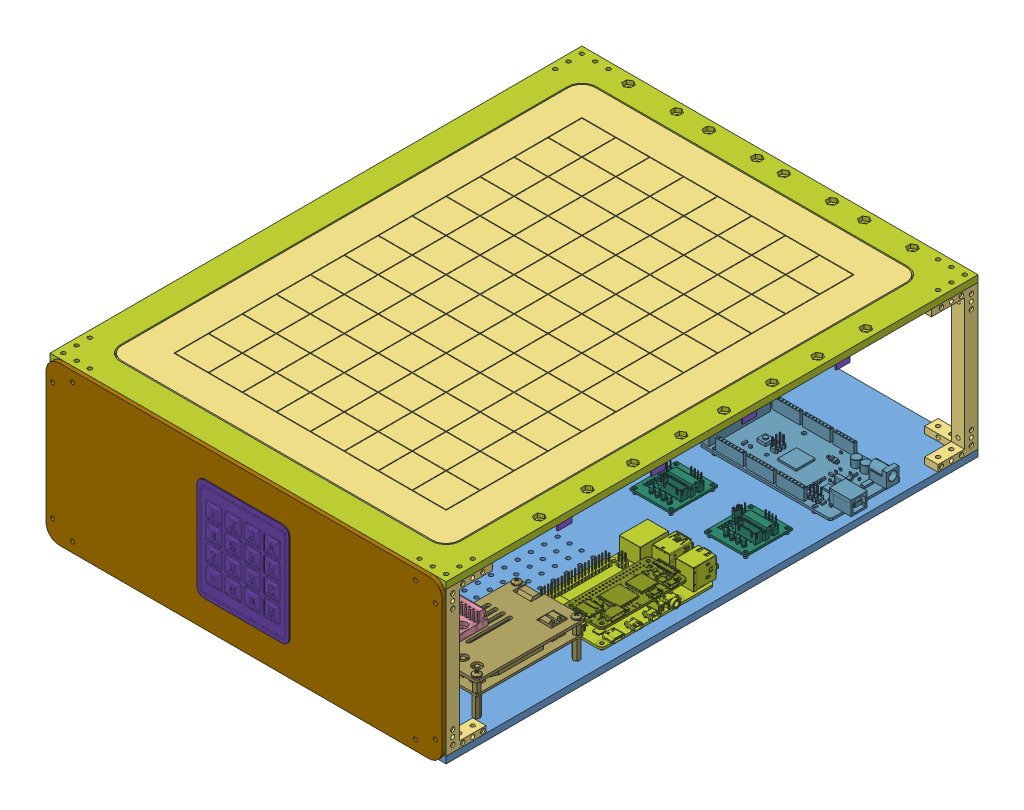
SolidWorks assembly FinalAssembly, configuration Default. Lengths in mm.
Overall size (297.5 118.5 403.99).
41 component instances, 27 part files, 115 mates.
Components (placement in the parent):
- Base-1: Base [Default] at (-28.1272 210.7626 518.1908) size (297.5 5 399.5)
- GearTrackLongAxisSinglePiece-1: GearTrackLongAxisSinglePiece [Default] at (155.3139 84.2058 503.2065) x (1 0 0) z (0 1 0) size (28 365.38 12.5)
- CornerJoin-1: CornerJoin [Default] at (-28.1272 215.7626 518.1908) size (35 108.5 35)
- CornerJoin-2: CornerJoin [Default] at (-28.1272 215.7626 118.6908) x (0 0 1) z (-1 0 0) size (35 108.5 35)
- CornerJoin-3: CornerJoin [Default] at (269.3728 215.7626 518.1908) x (0 0 -1) z (1 0 0) size (35 108.5 35)
- CornerJoin-4: CornerJoin [Default] at (269.3728 215.7626 118.6908) x (-1 0 0) z (0 0 -1) size (35 108.5 35)
- GearTrackShortAxisSinglePiece-1: GearTrackShortAxisSinglePiece [Default] at (251.3609 131.6956 442.9057) x (0 0 -1) z (0 1 0) size (28 245.31 12.5)
- AxisCartMount-1: AxisCartMount [Default] at (141.6223 251.1626 455.8667) x (-1 0 0) z (0 0 -1) size (154 5 33)
- ShortAxisLimitMount-1: ShortAxisLimitMount [Default] at (-19.5822 261.1626 458.0758) x (0 0 1) z (0 1 0) size (28 20 33)
- NewTopMount-1: NewTopMount [Default] at (-28.1272 324.2626 118.6908) x (0 0 1) z (-1 0 0) size (399.5 5 297.5)
- MotorCartMount-1: MotorCartMount [Default] at (63.6531 231.1626 374.4235) x (1 0 0) z (0 -1 0) size (44.96 33 30.65)
- MotorCartMount-2: MotorCartMount [Default] at (116.278 271.5626 415.1046) x (0 0 1) z (0 -1 0) size (44.96 33 30.65)
- EndEffectorMountV2-1: EndEffectorMountV2 [Default] at (1.8349 289.5626 493.0738) size (39 25 47)
- LCD_1602-1: LCD_1602 [Default] at (48.0597 363.4765 514.5115) x (1 0 0) z (0 -1 0) size (80 17 36)
- MagneticRod-1: MagneticRod [Default] at (18.3378 322.4583 471.3738) x (-1 0 0) z (0 0 1) size (5.8 23.9 5.8)
- ZK-JVA-12KX-1: ZK-JVA-12KX [Default] at (276.4205 168.0705 467.5621) x (0 0 -1) z (0 1 0) size (82 52 29.13)
- 28BYJ-48 5V Stepper Motor-1: 28BYJ-48 5V Stepper Motor [Default] at (120.624 250.1626 471.8089) x (1 0 0) z (0 -1 0) size (42 52.5 29)
- 28BYJ-48 5V Stepper Motor-2: 28BYJ-48 5V Stepper Motor [Default] at (18.8927 290.5626 472.0755) x (0 0 1) z (0 -1 0) size (42 52.5 29)
- ArduinoMega-1: ArduinoMega [Default] at (212.2228 219.4136 196.4827) x (1 0 0) z (0 -1 0) size (107.95 53.42 12.95)
- ULN2003-1: ULN2003 [Default] at (223.3728 217.7626 278.1908) x (1 0 0) z (0 1 0) size (31 35 11.29)
- ULN2003-2: ULN2003 [Default] at (167.3728 217.7626 278.1908) x (1 0 0) z (0 1 0) size (31 35 11.29)
- Raspberry Pi Zero 2 W-1: Raspberry Pi Zero 2 W [Default] at (246.3728 231.5626 360.6908) x (0 0 -1) z (1 0 0) size (65.8 5.05 30.58)
- keypad-16KeyMembrane-1: keypad-16KeyMembrane [Default] at (120.6223 270.0105 522.0036) x (1 0 0) z (0 -1 0) size (68.96 10.64 77.9)
- HK15178B-1: HK15178B [Default] at (24.2327 310.5583 503.0738) x (1 0 0) z (0 1 0) size (37.75 30.2 12)
- limit switch-1: limit switch [Default] at (-9.5822 279.1626 463.0758) x (-1 0 0) z (0 0 -1) size (26 20 11)
- limit switch-2: limit switch [Default] at (139.3728 240.7626 500.1908) x (0 0 1) z (-1 0 0) size (26 20 11)
- LongAxisLimitMount-1: LongAxisLimitMount [Default] at (134.3728 222.7626 510.1908) x (1 0 0) z (0 1 0) size (15 15 35)
- Board-2: Board [Default] at (-6.1272 326.2626 496.1908) size (253.5 3 355.5)
- RodAttach-1: RodAttach [Default] at (18.3378 322.5583 471.3738) x (0 0 1) z (1 0 0) size (14.5 24 9)
- LED-1: LED [Default] at (211.8357 326.4426 224.6643) x (0 0 -1) z (1 0 0) size (3.38 1.82 10.82)
- HallEffect-1: HallEffect [Default] at (207.8504 326.8526 230.6307) size (3.92 1.41 7.9)
- Raspberry Pi 4 Model B(CHIP SHORT REPLACEMENT)-1: Raspberry Pi 4 Model B(CHIP SHORT REPLACEMENT) [Default] at (233.3728 218.5626 350.6908) x (0 0 -1) z (1 0 0) size (89 19.92 58.4)
- 16ChannelMux-1: 16ChannelMux [Default] at (11.8728 324.2626 140.6908) x (0 0 -1) z (-1 0 0) size (17 9.94 40.4)
- 16ChannelMux-2: 16ChannelMux [Default] at (247.3728 324.2626 264.0908) x (1 0 0) z (0 0 -1) size (17 9.94 40.4)
- 16ChannelMux-3: 16ChannelMux [Default] at (72.2728 324.2626 140.6908) x (0 0 -1) z (-1 0 0) size (17 9.94 40.4)
- 16ChannelMux-4: 16ChannelMux [Default] at (128.5728 324.2626 140.6908) x (0 0 -1) z (-1 0 0) size (17 9.94 40.4)
- 16ChannelMux-5: 16ChannelMux [Default] at (247.3728 324.2626 402.7908) x (1 0 0) z (0 0 -1) size (17 9.94 40.4)
- 16ChannelMux-6: 16ChannelMux [Default] at (247.3728 324.2626 332.3908) x (1 0 0) z (0 0 -1) size (17 9.94 40.4)
- 16ChannelMux-7: 16ChannelMux [Default] at (247.3728 324.2626 193.6908) x (1 0 0) z (0 0 -1) size (17 9.94 40.4)
- 16ChannelMux-8: 16ChannelMux [Default] at (188.9728 324.2626 140.6908) x (0 0 -1) z (-1 0 0) size (17 9.94 40.4)
- InterfaceWall-1: InterfaceWall [Default] at (-28.1272 210.7626 518.1908) size (297.5 118.5 3)
Mates (geometry in assembly coordinates):
- Coincident1: coincident anti-aligned: plane of Base-1 through (-28.1272 215.7626 518.1908) normal (0 1 0); plane of GearTrackLongAxisSinglePiece-1 through (20.6226 215.7626 295.7853) normal (0 -1 0)
- Concentric1: concentric aligned: circle of Base-1; circle of GearTrackLongAxisSinglePiece-1
- Parallel2: parallel aligned: plane of Base-1 through (269.3728 215.7626 518.1908) normal (1 0 0); plane of GearTrackLongAxisSinglePiece-1 through (134.6203 215.7626 535.9174) normal (1 0 0)
- Coincident4: coincident anti-aligned: plane of Base-1 through (-28.1272 215.7626 518.1908) normal (0 1 0); plane of CornerJoin-1 through (-28.1272 215.7626 518.1908) normal (0 -1 0)
- Coincident6: coincident aligned: plane of Base-1 through (-28.1272 215.7626 518.1908) normal (0 0 1); plane of CornerJoin-1 through (-28.1272 225.7626 518.1908) normal (0 0 1)
- Coincident7: coincident aligned: plane of Base-1 through (-28.1272 215.7626 518.1908) normal (-1 0 0); plane of CornerJoin-1 through (-28.1272 225.7626 518.1908) normal (-1 0 0)
- Coincident8: coincident aligned: plane of Base-1 through (-28.1272 215.7626 518.1908) normal (-1 0 0); plane of CornerJoin-2 through (-28.1272 225.7626 118.6908) normal (-1 0 0)
- Coincident9: coincident anti-aligned: plane of Base-1 through (-28.1272 215.7626 518.1908) normal (0 1 0); plane of CornerJoin-2 through (-28.1272 215.7626 118.6908) normal (0 -1 0)
- Coincident10: coincident aligned: plane of Base-1 through (-28.1272 215.7626 118.6908) normal (0 0 -1); plane of CornerJoin-2 through (-28.1272 225.7626 118.6908) normal (0 0 -1)
- Coincident11: coincident anti-aligned: plane of Base-1 through (-28.1272 215.7626 518.1908) normal (0 1 0); plane of CornerJoin-3 through (269.3728 215.7626 518.1908) normal (0 -1 0)
- Coincident12: coincident aligned: plane of Base-1 through (-28.1272 215.7626 518.1908) normal (0 0 1); plane of CornerJoin-3 through (269.3728 225.7626 518.1908) normal (0 0 1)
- Coincident13: coincident aligned: plane of Base-1 through (269.3728 215.7626 518.1908) normal (1 0 0); plane of CornerJoin-3 through (269.3728 225.7626 518.1908) normal (1 0 0)
- Coincident14: coincident anti-aligned: plane of Base-1 through (-28.1272 215.7626 518.1908) normal (0 1 0); plane of CornerJoin-4 through (269.3728 215.7626 118.6908) normal (0 -1 0)
- Coincident15: coincident aligned: plane of Base-1 through (-28.1272 215.7626 118.6908) normal (0 0 -1); plane of CornerJoin-4 through (269.3728 225.7626 118.6908) normal (0 0 -1)
- Coincident16: coincident aligned: plane of Base-1 through (269.3728 215.7626 518.1908) normal (1 0 0); plane of CornerJoin-4 through (269.3728 225.7626 118.6908) normal (1 0 0)
- Coincident17: coincident anti-aligned: plane of CornerJoin-1 through (-28.1272 324.2626 518.1908) normal (0 1 0); plane of NewTopMount-1 through (-28.1272 324.2626 118.6908) normal (0 -1 0)
- Coincident18: coincident aligned: plane of CornerJoin-3 through (269.3728 225.7626 518.1908) normal (0 0 1); plane of NewTopMount-1 through (-28.1272 329.2626 518.1908) normal (0 0 1)
- Coincident19: coincident aligned: plane of CornerJoin-3 through (269.3728 225.7626 518.1908) normal (1 0 0); plane of NewTopMount-1 through (269.3728 329.2626 118.6908) normal (1 0 0)
- Coincident24: coincident anti-aligned: plane of GearTrackLongAxisSinglePiece-1 through (20.6226 228.2626 535.9174) normal (0 1 0); plane of MotorCartMount-1 through (63.6531 228.2626 374.4235) normal (0 -1 0)
- Distance3: distance = 7 mm aligned: plane of GearTrackLongAxisSinglePiece-1 through (106.6223 215.7626 535.9174) normal (-1 0 0); plane of MotorCartMount-1 through (99.6223 231.1626 374.4235) normal (-1 0 0)
- Coincident26: coincident anti-aligned: plane of AxisCartMount-1 through (141.6223 251.1626 455.8667) normal (0 -1 0); plane of MotorCartMount-1 through (63.6531 251.1626 374.4235) normal (0 1 0)
- Coincident27: coincident aligned: plane of AxisCartMount-1 through (141.6223 256.1626 455.8667) normal (0 0 -1); plane of MotorCartMount-1 through (63.6531 231.1626 455.8667) normal (0 0 -1)
- Concentric2: concentric aligned: cylinder of AxisCartMount-1 through (137.8723 247.1626 460.3667) axis (0 1 0) radius 1.65; cylinder of MotorCartMount-1 through (137.8723 212.1626 460.3667) axis (0 1 0) radius 1.65
- Coincident29: coincident anti-aligned: plane of GearTrackShortAxisSinglePiece-1 through (0.5498 256.1626 486.0738) normal (0 -1 0); plane of AxisCartMount-1 through (141.6223 256.1626 455.8667) normal (0 1 0)
- Concentric5: concentric aligned: circle of GearTrackShortAxisSinglePiece-1; circle of AxisCartMount-1
- Parallel5: parallel aligned: plane of GearTrackShortAxisSinglePiece-1 through (0.5498 260.9126 486.0738) normal (0 0 1); plane of AxisCartMount-1 through (141.6223 256.1626 488.8667) normal (0 0 1)
- Coincident34: coincident anti-aligned: plane of GearTrackShortAxisSinglePiece-1 through (0.4178 256.1626 572.0736) normal (-1 0 0); plane of ShortAxisLimitMount-1 through (0.4178 261.1626 458.0758) normal (1 0 0)
- Coincident35: coincident aligned: plane of GearTrackShortAxisSinglePiece-1 through (157.8602 256.1626 572.0736) normal (0 -1 0); plane of ShortAxisLimitMount-1 through (0.4178 256.1626 458.0758) normal (0 -1 0)
- Coincident36: coincident aligned: plane of GearTrackShortAxisSinglePiece-1 through (0.5498 260.9126 458.0758) normal (0 0 -1); plane of ShortAxisLimitMount-1 through (0.4178 261.1626 458.0758) normal (0 0 -1)
- Coincident38: coincident anti-aligned: plane of GearTrackShortAxisSinglePiece-1 through (277.9263 268.6626 572.0736) normal (0 1 0); plane of MotorCartMount-2 through (116.278 268.6626 415.1046) normal (0 -1 0)
- Distance4: distance = 7 mm aligned: plane of MotorCartMount-2 through (116.278 271.5626 493.0738) normal (0 0 1); plane of GearTrackShortAxisSinglePiece-1 through (0.5498 260.9126 486.0738) normal (0 0 1)
- Coincident40: coincident anti-aligned: plane of MotorCartMount-2 through (116.278 291.5626 415.1046) normal (0 1 0); plane of EndEffectorMountV2-1 through (38.8349 291.5626 487.5831) normal (0 -1 0)
- Concentric6: concentric anti-aligned: circle of MotorCartMount-2; circle of EndEffectorMountV2-1
- Coincident42: coincident aligned: plane of MotorCartMount-2 through (34.8349 271.5626 415.1046) normal (1 0 0); plane of EndEffectorMountV2-1 through (34.8349 294.5626 493.0738) normal (1 0 0)
- Coincident43: coincident anti-aligned: plane of EndEffectorMountV2-1 through (12.5349 321.9709 492.5738) normal (0 0 -1); plane of HK15178B-1 through (24.2327 310.5583 492.5738) normal (0 0 1)
- Concentric7: concentric aligned: circle of EndEffectorMountV2-1; circle of HK15178B-1
- Parallel6: parallel anti-aligned: plane of EndEffectorMountV2-1 through (1.8349 304.5626 493.0738) normal (0 1 0); plane of HK15178B-1 through (12.7327 304.5583 492.5738) normal (0 -1 0)
- Concentric8: concentric aligned: circle of MotorCartMount-1; cylinder of 28BYJ-48 5V Stepper Motor-1 through (120.624 227.1626 463.8089) axis (0 1 0) radius 2.5
- Parallel7: parallel aligned: plane of MotorCartMount-1 through (63.6531 231.1626 488.8667) normal (0 0 1); plane of 28BYJ-48 5V Stepper Motor-1 through (129.424 246.1626 490.3089) normal (0 0 1)
- Coincident45: coincident anti-aligned: plane of MotorCartMount-1 through (63.6531 231.1626 374.4235) normal (0 1 0); plane of 28BYJ-48 5V Stepper Motor-1 through (120.624 231.1626 471.8089) normal (0 -1 0)
- Concentric11: concentric aligned: circle of MotorCartMount-2; cylinder of 28BYJ-48 5V Stepper Motor-2 through (26.8927 267.5626 472.0755) axis (0 1 0) radius 2.5
- Parallel8: parallel aligned: plane of MotorCartMount-2 through (1.8349 271.5626 415.1046) normal (-1 0 0); plane of 28BYJ-48 5V Stepper Motor-2 through (0.3927 286.5626 480.8755) normal (-1 0 0)
- Coincident47: coincident anti-aligned: plane of MotorCartMount-2 through (116.278 271.5626 415.1046) normal (0 1 0); plane of 28BYJ-48 5V Stepper Motor-2 through (18.8927 271.5626 472.0755) normal (0 -1 0)
- Coincident48: coincident aligned: circle of ShortAxisLimitMount-1; circle of limit switch-1
- Concentric12: concentric aligned: circle of ShortAxisLimitMount-1; circle of limit switch-1
- Distance6: distance = 29 mm anti-aligned: plane of limit switch-2 through (131.3728 248.7626 489.1908) normal (0 0 -1); plane of Base-1 through (-28.1272 215.7626 518.1908) normal (0 0 1)
- Distance7: distance = 15 mm anti-aligned: plane of Base-1 through (-28.1272 215.7626 518.1908) normal (0 1 0); plane of limit switch-2 through (137.3728 230.7626 490.1908) normal (0 -1 0)
- Distance8: distance = 130 mm aligned: plane of limit switch-2 through (139.3728 240.7626 500.1908) normal (1 0 0); plane of Base-1 through (269.3728 215.7626 518.1908) normal (1 0 0)
- Coincident55: coincident anti-aligned: plane of Base-1 through (-28.1272 215.7626 518.1908) normal (0 1 0); plane of LongAxisLimitMount-1 through (134.3728 215.7626 510.1908) normal (0 -1 0)
- Coincident57: coincident anti-aligned: plane of limit switch-2 through (139.3728 240.7626 500.1908) normal (1 0 0); plane of LongAxisLimitMount-1 through (139.3728 250.7626 510.1908) normal (-1 0 0)
- Coincident60: coincident aligned: plane of limit switch-2 through (137.3728 230.7626 510.1908) normal (0 0 1); plane of LongAxisLimitMount-1 through (134.3728 222.7626 510.1908) normal (0 0 1)
- Coincident61: coincident anti-aligned: plane of NewTopMount-1 through (3.8728 326.2626 486.1908) normal (0 1 0); plane of Board-2 through (-6.1272 326.2626 496.1908) normal (0 -1 0)
- Coincident62: coincident anti-aligned: plane of NewTopMount-1 through (3.8728 326.2626 486.1908) normal (0 1 0); plane of Board-2 through (-6.1272 326.2626 496.1908) normal (0 -1 0)
- Distance9: distance = 1 mm anti-aligned: plane of Board-2 through (247.3728 329.2626 496.1908) normal (1 0 0); plane of NewTopMount-1 through (248.3728 326.2626 150.6908) normal (-1 0 0)
- Distance10: distance = 1 mm anti-aligned: plane of Board-2 through (-6.1272 329.2626 140.6908) normal (0 0 -1); plane of NewTopMount-1 through (237.3728 326.2626 139.6908) normal (0 0 1)
- Concentric15: concentric aligned: circle of MagneticRod-1; circle of RodAttach-1
- Coincident65: coincident aligned: plane of MagneticRod-1 through (18.3378 298.5583 471.3738) normal (0 -1 0); plane of RodAttach-1 through (18.3378 298.5583 471.3738) normal (0 -1 0)
- Concentric16: concentric aligned: circle of HK15178B-1; circle of RodAttach-1
- Coincident66: coincident anti-aligned: plane of HK15178B-1 through (21.6452 310.5583 481.3738) normal (0 0 -1); plane of RodAttach-1 through (18.3378 298.5583 481.3738) normal (0 0 1)
- Parallel9: parallel aligned: plane of EndEffectorMountV2-1 through (1.8349 294.5626 493.0738) normal (0 1 0); plane of RodAttach-1 through (18.3378 322.5583 471.3738) normal (0 1 0)
- Coincident68: coincident anti-aligned: plane of Board-2 through (-6.1272 328.2626 496.1908) normal (0 -1 0); plane of HallEffect-1 through (207.8504 328.2626 230.6307) normal (0 1 0)
- Coincident69: coincident anti-aligned: plane of Board-2 through (-6.1272 328.2626 496.1908) normal (0 -1 0); plane of LED-1 through (211.8357 328.2626 224.6643) normal (0 1 0)
- Parallel10: parallel anti-aligned: plane of Board-2 through (-6.1272 328.2626 220.8108) normal (0 0 1); plane of LED-1 through (211.8357 328.2626 221.2843) normal (0 0 -1)
- Coincident72: coincident anti-aligned: plane of Base-1 through (-28.1272 215.7626 518.1908) normal (0 1 0); plane of ZK-JVA-12KX-1 through (207.2747 215.7626 405.6908) normal (0 -1 0)
- Parallel11: parallel anti-aligned: plane of Base-1 through (-28.1272 215.7626 518.1908) normal (0 0 1); plane of ZK-JVA-12KX-1 through (257.3728 232.3626 403.1908) normal (0 0 -1)
- Distance12: distance = 35 mm aligned: plane of ZK-JVA-12KX-1 through (257.3728 232.3626 483.1908) normal (0 0 1); plane of Base-1 through (-28.1272 215.7626 518.1908) normal (0 0 1)
- Distance13: distance = 12 mm aligned: plane of ZK-JVA-12KX-1 through (257.3728 232.3626 403.1908) normal (1 0 0); plane of Base-1 through (269.3728 215.7626 518.1908) normal (1 0 0)
- Parallel12: parallel aligned: plane of Base-1 through (269.3728 215.7626 518.1908) normal (1 0 0); plane of Raspberry Pi 4 Model B(CHIP SHORT REPLACEMENT)-1 through (261.3728 219.3626 393.1908) normal (1 0 0)
- Parallel13: parallel anti-aligned: plane of Base-1 through (-28.1272 215.7626 518.1908) normal (0 1 0); plane of Raspberry Pi 4 Model B(CHIP SHORT REPLACEMENT)-1 through (233.3728 217.7626 350.6908) normal (0 -1 0)
- Distance14: distance = 8 mm aligned: plane of Raspberry Pi 4 Model B(CHIP SHORT REPLACEMENT)-1 through (261.3728 219.3626 393.1908) normal (1 0 0); plane of Base-1 through (269.3728 215.7626 518.1908) normal (1 0 0)
- Distance15: distance = 125 mm aligned: plane of Raspberry Pi 4 Model B(CHIP SHORT REPLACEMENT)-1 through (205.3728 219.3626 393.1908) normal (0 0 1); plane of Base-1 through (-28.1272 215.7626 518.1908) normal (0 0 1)
- Distance16: distance = 2 mm anti-aligned: plane of Raspberry Pi 4 Model B(CHIP SHORT REPLACEMENT)-1 through (233.3728 217.7626 350.6908) normal (0 -1 0); plane of Base-1 through (-28.1272 215.7626 518.1908) normal (0 1 0)
- Coincident85: coincident aligned: plane of Raspberry Pi Zero 2 W-1 through (231.3728 232.3626 393.1908) normal (0 0 1); plane of Raspberry Pi 4 Model B(CHIP SHORT REPLACEMENT)-1 through (205.3728 219.3626 393.1908) normal (0 0 1)
- Coincident87: coincident aligned: plane of Raspberry Pi Zero 2 W-1 through (261.3728 232.3626 393.1908) normal (1 0 0); plane of Raspberry Pi 4 Model B(CHIP SHORT REPLACEMENT)-1 through (261.3728 219.3626 393.1908) normal (1 0 0)
- Distance18: distance = 15 mm anti-aligned: plane of Raspberry Pi Zero 2 W-1 through (246.3728 230.7626 360.6908) normal (0 -1 0); plane of Base-1 through (-28.1272 215.7626 518.1908) normal (0 1 0)
- Coincident89: coincident aligned: plane of Base-1 through (269.3728 215.7626 518.1908) normal (1 0 0); plane of ArduinoMega-1 through (269.3728 230.2086 213.9198) normal (1 0 0)
- Distance19: distance = 2 mm anti-aligned: plane of ArduinoMega-1 through (263.0228 217.7626 169.7746) normal (0 -1 0); plane of Base-1 through (-28.1272 215.7626 518.1908) normal (0 1 0)
- Distance20: distance = 2 mm anti-aligned: plane of ULN2003-2 through (167.3728 217.7626 278.1908) normal (0 -1 0); plane of Base-1 through (-28.1272 215.7626 518.1908) normal (0 1 0)
- Distance21: distance = 2 mm anti-aligned: plane of ULN2003-1 through (223.3728 217.7626 278.1908) normal (0 -1 0); plane of Base-1 through (-28.1272 215.7626 518.1908) normal (0 1 0)
- Coincident90: coincident anti-aligned: plane of NewTopMount-1 through (-28.1272 324.2626 118.6908) normal (0 -1 0); plane of 16ChannelMux-1 through (11.8728 324.2626 140.6908) normal (0 1 0)
- Distance22: distance = 5 mm aligned: plane of 16ChannelMux-1 through (11.8728 322.8226 123.6908) normal (0 0 -1); plane of NewTopMount-1 through (-28.1272 329.2626 118.6908) normal (0 0 -1)
- Coincident92: coincident anti-aligned: plane of NewTopMount-1 through (-28.1272 324.2626 118.6908) normal (0 -1 0); plane of 16ChannelMux-3 through (72.2728 324.2626 140.6908) normal (0 1 0)
- Coincident93: coincident aligned: plane of 16ChannelMux-1 through (11.8728 322.8226 123.6908) normal (0 0 -1); plane of 16ChannelMux-3 through (72.2728 322.8226 123.6908) normal (0 0 -1)
- Coincident94: coincident anti-aligned: plane of NewTopMount-1 through (-28.1272 324.2626 118.6908) normal (0 -1 0); plane of 16ChannelMux-4 through (128.5728 324.2626 140.6908) normal (0 1 0)
- Coincident95: coincident aligned: plane of 16ChannelMux-3 through (72.2728 322.8226 123.6908) normal (0 0 -1); plane of 16ChannelMux-4 through (128.5728 322.8226 123.6908) normal (0 0 -1)
- Coincident96: coincident anti-aligned: plane of NewTopMount-1 through (-28.1272 324.2626 118.6908) normal (0 -1 0); plane of 16ChannelMux-8 through (188.9728 324.2626 140.6908) normal (0 1 0)
- Coincident97: coincident aligned: plane of 16ChannelMux-4 through (128.5728 322.8226 123.6908) normal (0 0 -1); plane of 16ChannelMux-8 through (188.9728 322.8226 123.6908) normal (0 0 -1)
- Distance23: distance = 5 mm anti-aligned: plane of CornerJoin-4 through (234.3728 215.7626 118.6908) normal (-1 0 0); plane of 16ChannelMux-8 through (229.3728 322.8226 140.6908) normal (1 0 0)
- Distance24: distance = 5 mm anti-aligned: plane of CornerJoin-2 through (6.8728 215.7626 118.6908) normal (1 0 0); plane of 16ChannelMux-1 through (11.8728 322.8226 140.6908) normal (-1 0 0)
- Distance25: distance = 20 mm anti-aligned: plane of 16ChannelMux-4 through (168.9728 322.8226 140.6908) normal (1 0 0); plane of 16ChannelMux-8 through (188.9728 322.8226 140.6908) normal (-1 0 0)
- Distance26: distance = 20 mm anti-aligned: plane of 16ChannelMux-1 through (52.2728 322.8226 140.6908) normal (1 0 0); plane of 16ChannelMux-3 through (72.2728 322.8226 140.6908) normal (-1 0 0)
- Coincident105: coincident anti-aligned: plane of NewTopMount-1 through (-28.1272 324.2626 118.6908) normal (0 -1 0); plane of 16ChannelMux-7 through (247.3728 324.2626 193.6908) normal (0 1 0)
- Distance27: distance = 5 mm aligned: plane of 16ChannelMux-7 through (264.3728 322.8226 193.6908) normal (1 0 0); plane of NewTopMount-1 through (269.3728 329.2626 118.6908) normal (1 0 0)
- Coincident107: coincident anti-aligned: plane of NewTopMount-1 through (-28.1272 324.2626 118.6908) normal (0 -1 0); plane of 16ChannelMux-2 through (247.3728 324.2626 264.0908) normal (0 1 0)
- Coincident108: coincident anti-aligned: plane of NewTopMount-1 through (-28.1272 324.2626 118.6908) normal (0 -1 0); plane of 16ChannelMux-6 through (247.3728 324.2626 332.3908) normal (0 1 0)
- Coincident109: coincident anti-aligned: plane of NewTopMount-1 through (-28.1272 324.2626 118.6908) normal (0 -1 0); plane of 16ChannelMux-5 through (247.3728 324.2626 402.7908) normal (0 1 0)
- Coincident110: coincident aligned: plane of 16ChannelMux-2 through (264.3728 322.8226 264.0908) normal (1 0 0); plane of 16ChannelMux-7 through (264.3728 322.8226 193.6908) normal (1 0 0)
- Coincident111: coincident aligned: plane of 16ChannelMux-2 through (264.3728 322.8226 264.0908) normal (1 0 0); plane of 16ChannelMux-6 through (264.3728 322.8226 332.3908) normal (1 0 0)
- Coincident112: coincident aligned: plane of 16ChannelMux-5 through (264.3728 322.8226 402.7908) normal (1 0 0); plane of 16ChannelMux-6 through (264.3728 322.8226 332.3908) normal (1 0 0)
- Distance28: distance = 40 mm anti-aligned: plane of 16ChannelMux-5 through (247.3728 322.8226 443.1908) normal (0 0 1); plane of CornerJoin-3 through (269.3728 215.7626 483.1908) normal (0 0 -1)
- Distance29: distance = 40 mm anti-aligned: plane of CornerJoin-4 through (269.3728 215.7626 153.6908) normal (0 0 1); plane of 16ChannelMux-7 through (247.3728 322.8226 193.6908) normal (0 0 -1)
- Distance31: distance = 30 mm anti-aligned: plane of 16ChannelMux-6 through (247.3728 322.8226 372.7908) normal (0 0 1); plane of 16ChannelMux-5 through (247.3728 322.8226 402.7908) normal (0 0 -1)
- Distance32: distance = 30 mm anti-aligned: plane of 16ChannelMux-7 through (247.3728 322.8226 234.0908) normal (0 0 1); plane of 16ChannelMux-2 through (247.3728 322.8226 264.0908) normal (0 0 -1)
- Coincident122: coincident aligned: plane of NewTopMount-1 through (-28.1272 329.2626 118.6908) normal (0 1 0); plane of InterfaceWall-1 through (-28.1272 329.2626 521.1908) normal (0 1 0)
- Coincident123: coincident aligned: plane of CornerJoin-1 through (-28.1272 225.7626 518.1908) normal (-1 0 0); plane of InterfaceWall-1 through (-28.1272 210.7626 521.1908) normal (-1 0 0)
- Coincident124: coincident anti-aligned: plane of CornerJoin-1 through (-28.1272 225.7626 518.1908) normal (0 0 1); plane of InterfaceWall-1 through (-28.1272 210.7626 518.1908) normal (0 0 -1)
- Coincident125: coincident anti-aligned: plane of keypad-16KeyMembrane-1 through (120.6223 270.0105 521.1908) normal (0 0 -1); plane of InterfaceWall-1 through (-28.1272 210.7626 521.1908) normal (0 0 1)
- Distance34: distance = 114.27 mm aligned: plane of keypad-16KeyMembrane-1 through (155.1028 236.6476 522.0036) normal (1 0 0); plane of InterfaceWall-1 through (269.3728 210.7626 521.1908) normal (1 0 0)
- Distance35: distance = 20.805 mm aligned: plane of keypad-16KeyMembrane-1 through (91.2218 231.5676 522.0036) normal (0 -1 0); plane of InterfaceWall-1 through (-28.1272 210.7626 521.1908) normal (0 -1 0)
- Coincident130: coincident aligned: plane of LCD_1602-1 through (9.0088 270.8765 521.1908) normal (0 0 1); plane of InterfaceWall-1 through (-28.1272 210.7626 521.1908) normal (0 0 1)
- Coincident131: coincident aligned: plane of ULN2003-1 through (223.3728 217.7626 278.1908) normal (0 0 1); plane of ULN2003-2 through (167.3728 217.7626 278.1908) normal (0 0 1)
- Distance36: distance = 25 mm anti-aligned: plane of ULN2003-2 through (198.3728 217.7626 278.1908) normal (1 0 0); plane of ULN2003-1 through (223.3728 217.7626 243.1908) normal (-1 0 0)
- Distance37: distance = 15 mm aligned: plane of ULN2003-1 through (254.3728 217.7626 278.1908) normal (1 0 0); plane of Base-1 through (269.3728 215.7626 518.1908) normal (1 0 0)
- Distance38: distance = 30 mm anti-aligned: plane of ULN2003-1 through (223.3728 217.7626 278.1908) normal (0 0 1); plane of Raspberry Pi 4 Model B(CHIP SHORT REPLACEMENT)-1 through (205.3728 219.3626 308.1908) normal (0 0 -1)
- Distance39: distance = 20 mm anti-aligned: plane of ArduinoMega-1 through (161.4228 217.7626 223.1908) normal (0 0 1); plane of ULN2003-1 through (254.3728 217.7626 243.1908) normal (0 0 -1)
